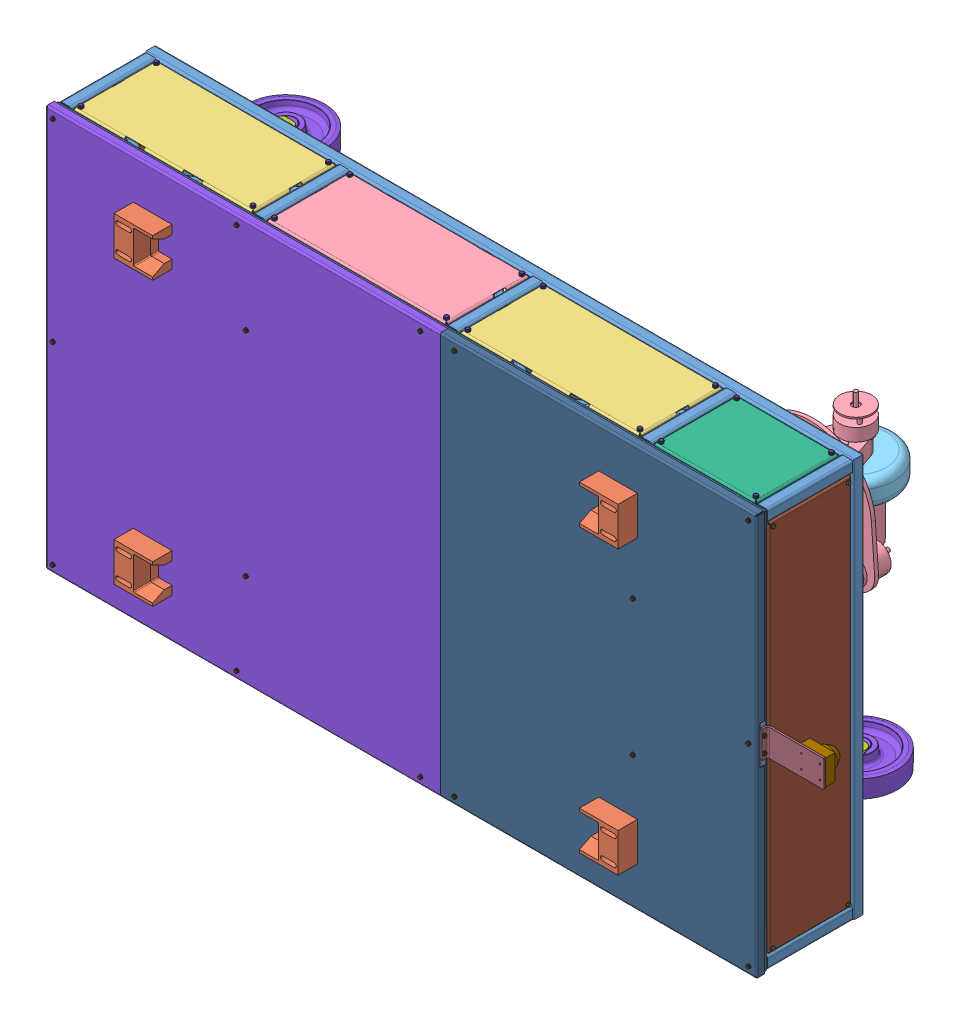
SolidWorks assembly spartaco_bot_V1, configuration Default. Lengths in mm.
Overall size (1986.1 1042.2 588.68).
206 component instances, 48 part files, 27 mates.
Components (placement in the parent):
- robot_body-1: robot_body [Default] at (-881.7629 -500.0018 -180.7451) x (0 -1 0) z (-1 0 0) size (1042.2 351.5 1986.1)
  - 00-A-PT0046 (1).step-1: 00-A-PT0046 (1).step [Default] at origin size (1042.2 306.3 1986.1)
    - 00-P-PT0151_Default_A macchina_.step-1: 00-P-PT0151_Default_A macchina_.step [Default] at origin size (1030 285 1830)
    - 00-P-PT0177.step-1: 00-P-PT0177.step [Default] at (-500 125 15) size (965 215 15)
    - 00-P-PT0153.step-1: 00-P-PT0153.step [Default] at (-1015 125 -250) x (0 0 1) z (-1 0 0) size (465 215 15)
    - 00-P-PT0153.step-2: 00-P-PT0153.step [Default] at (15 125 -250) x (0 0 -1) z (1 0 0) size (465 215 15)
    - 00-P-PT0153.step-3: 00-P-PT0153.step [Default] at (15 125 -1250) x (0 0 -1) z (1 0 0) size (465 215 15)
    - 00-P-PT0153.step-4: 00-P-PT0153.step [Default] at (-1015 125 -1250) x (0 0 1) z (-1 0 0) size (465 215 15)
    - 00-P-PT0169.step-1: 00-P-PT0169.step [Default] at (-1015 125 -750) x (0 0 1) z (-1 0 0) size (465 215 15)
    - 00-P-PT0154.step-1: 00-P-PT0154.step [Default] at (-500 -35 -750) x (0 0 1) z (-1 0 0) size (525 53 557)
    - 00-P-PT0168.step-1: 00-P-PT0168.step [Default] at (15 125 -1650) x (0 0 -1) z (1 0 0) size (265 215 15)
    - 00-P-PT0168.step-2: 00-P-PT0168.step [Default] at (-1015 125 -1650) x (0 0 1) z (-1 0 0) size (265 215 15)
    - 00-A-PT0167.step-1: 00-A-PT0167.step [Default] at (-500 -31 -590) size (500 35 45)
    - 00-P-PT0169.step-2: 00-P-PT0169.step [Default] at (15 125 -750) x (0 0 -1) z (1 0 0) size (465 215 15)
    - 00-A-PT0167.step-2: 00-A-PT0167.step [Default] at (-500 -31 -910) x (-1 0 0) z (0 0 -1) size (500 35 45)
    - 00-P-PT0174.step-1: 00-P-PT0174.step [Default] at (-500 266.5 -899.5) x (0 0 1) z (-1 0 0) size (1020 20 1038.01)
    - 00-P-PT0173.step-1: 00-P-PT0173.step [Default] at (-25 15 -990) x (0 0 1) z (1 0 0) size (500 2 950)
    - 00-P-PT0171.step-1: 00-P-PT0171.step [Default] at (-500 266.5 -899.5) x (0 0 -1) z (1 0 0) size (818 20 1038.01)
    - 00-p-pt0152.step-1: 00-p-pt0152.step [Default] at (-500 125 -1815) x (-1 0 0) z (0 0 -1) size (965 215 15)
    - 00-P-PT0175.step-1: 00-P-PT0175.step [Default] at (-25 17 -505) x (0 0 -1) z (1 0 0) size (190 2 950)
    - 00-p-pt0176.step-1: 00-p-pt0176.step [Default] at (-535 234.8 -1815) size (70 20 150)
    - Rosetta Piana UNI6592_130909006.step-1: Rosetta Piana UNI6592_130909006.step [Default] at (-1015.8 27.5 -1527.5) x (0 -1 0) z (0 0 1) size (11 1.6 11)
    - Rosetta Piana UNI6592_130909006.step-2: Rosetta Piana UNI6592_130909006.step [Default] at (-1015.8 222.5 -1527.5) x (0 -1 0) z (0 0 1) size (11 1.6 11)
    - Rosetta Piana UNI6592_130909006.step-3: Rosetta Piana UNI6592_130909006.step [Default] at (-1015.8 222.5 -1772.5) x (0 -1 0) z (0 0 1) size (11 1.6 11)
    - Rosetta Piana UNI6592_130909006.step-4: Rosetta Piana UNI6592_130909006.step [Default] at (-1015.8 27.5 -1772.5) x (0 -1 0) z (0 0 1) size (11 1.6 11)
    - Rosetta Piana UNI6592_130909006.step-5: Rosetta Piana UNI6592_130909006.step [Default] at (-1015.8 27.5 -1472.5) x (0 -1 0) z (0 0 1) size (11 1.6 11)
    - Rosetta Piana UNI6592_130909006.step-6: Rosetta Piana UNI6592_130909006.step [Default] at (-1015.8 27.5 -1027.5) x (0 0 -1) z (0 -1 0) size (11 1.6 11)
    - Rosetta Piana UNI6592_130909006.step-7: Rosetta Piana UNI6592_130909006.step [Default] at (-1015.8 222.5 -972.5) x (0 -1 0) z (0 0 1) size (11 1.6 11)
    - Rosetta Piana UNI6592_130909006.step-8: Rosetta Piana UNI6592_130909006.step [Default] at (-1015.8 222.5 -527.5) x (0 -1 0) z (0 0 1) size (11 1.6 11)
    - Rosetta Piana UNI6592_130909006.step-9: Rosetta Piana UNI6592_130909006.step [Default] at (-1015.8 27.5 -472.5) x (0 -1 0) z (0 0 1) size (11 1.6 11)
    - Rosetta Piana UNI6592_130909006.step-10: Rosetta Piana UNI6592_130909006.step [Default] at (-1015.8 27.5 -27.5) x (0 -1 0) z (0 0 1) size (11 1.6 11)
    - Rosetta Piana UNI6592_130909006.step-11: Rosetta Piana UNI6592_130909006.step [Default] at (-972.5 222.5 0.6) x (1 0 0) z (0 1 0) size (11 1.6 11)
    - Rosetta Piana UNI6592_130909006.step-12: Rosetta Piana UNI6592_130909006.step [Default] at (-972.5 27.5 15.8) x (1 0 0) z (0 1 0) size (11 1.6 11)
    - Rosetta Piana UNI6592_130909006.step-13: Rosetta Piana UNI6592_130909006.step [Default] at (-27.5 27.5 15.8) x (1 0 0) z (0 1 0) size (11 1.6 11)
    - Rosetta Piana UNI6592_130909006.step-14: Rosetta Piana UNI6592_130909006.step [Default] at (15.8 27.5 -27.5) x (0 1 0) z (0 0 1) size (11 1.6 11)
    - Rosetta Piana UNI6592_130909006.step-15: Rosetta Piana UNI6592_130909006.step [Default] at (15.8 27.5 -472.5) x (0 1 0) z (0 0 1) size (11 1.6 11)
    - Rosetta Piana UNI6592_130909006.step-16: Rosetta Piana UNI6592_130909006.step [Default] at (15.8 222.5 -527.5) x (0 1 0) z (0 0 1) size (11 1.6 11)
    - Rosetta Piana UNI6592_130909006.step-17: Rosetta Piana UNI6592_130909006.step [Default] at (15.8 222.5 -972.5) x (0 1 0) z (0 0 1) size (11 1.6 11)
    - Rosetta Piana UNI6592_130909006.step-18: Rosetta Piana UNI6592_130909006.step [Default] at (15.8 27.5 -1027.5) x (0 1 0) z (0 0 1) size (11 1.6 11)
    - Rosetta Piana UNI6592_130909006.step-19: Rosetta Piana UNI6592_130909006.step [Default] at (15.8 27.5 -1472.5) x (0 1 0) z (0 0 1) size (11 1.6 11)
    - Rosetta Piana UNI6592_130909006.step-20: Rosetta Piana UNI6592_130909006.step [Default] at (15.8 27.5 -1527.5) x (0 1 0) z (0 0 1) size (11 1.6 11)
    - Rosetta Piana UNI6592_130909006.step-21: Rosetta Piana UNI6592_130909006.step [Default] at (15.8 27.5 -1772.5) x (0 1 0) z (0 0 1) size (11 1.6 11)
    - Rosetta Piana UNI6592_130909006.step-22: Rosetta Piana UNI6592_130909006.step [Default] at (15.8 222.5 -1527.5) x (0 1 0) z (0 0 1) size (11 1.6 11)
    - Rosetta Piana UNI6592_130909006.step-23: Rosetta Piana UNI6592_130909006.step [Default] at (15.8 222.5 -1772.5) x (0 1 0) z (0 0 1) size (11 1.6 11)
    - Rosetta Piana UNI6592_130909005.step-1: Rosetta Piana UNI6592_130909005.step [Default] at (-27.5 27.5 -1815.4) x (1 0 0) z (0 -1 0) size (10 0.8 10)
    - Rosetta Piana UNI6592_130909005.step-2: Rosetta Piana UNI6592_130909005.step [Default] at (-27.5 222.5 -1815.4) x (1 0 0) z (0 -1 0) size (10 0.8 10)
    - Rosetta Piana UNI6592_130909005.step-3: Rosetta Piana UNI6592_130909005.step [Default] at (-972.5 27.5 -1815.4) x (1 0 0) z (0 -1 0) size (10 0.8 10)
    - Rosetta Piana UNI6592_130909005.step-4: Rosetta Piana UNI6592_130909005.step [Default] at (-972.5 222.5 -1815.4) x (1 0 0) z (0 -1 0) size (10 0.8 10)
    - Rosetta Piana UNI6592_130909005.step-5: Rosetta Piana UNI6592_130909005.step [Default] at (-750 18.4 -500) x (0.837169 0 0.546944) z (0.546944 0 -0.837169) size (10 0.8 10)
    - Rosetta Piana UNI6592_130909005.step-6: Rosetta Piana UNI6592_130909005.step [Default] at (-500 18.4 -500) x (0.837169 0 0.546944) z (0.546944 0 -0.837169) size (10 0.8 10)
    - Rosetta Piana UNI6592_130909005.step-7: Rosetta Piana UNI6592_130909005.step [Default] at (-250 18.4 -500) x (0.837169 0 0.546944) z (0.546944 0 -0.837169) size (10 0.8 10)
    - Rosetta Piana UNI6592_130909005.step-8: Rosetta Piana UNI6592_130909005.step [Default] at (-250 18.4 -1000) x (0.837169 0 0.546944) z (0.546944 0 -0.837169) size (10 0.8 10)
    - Rosetta Piana UNI6592_130909005.step-9: Rosetta Piana UNI6592_130909005.step [Default] at (-500 18.4 -1000) x (0.837169 0 0.546944) z (0.546944 0 -0.837169) size (10 0.8 10)
    - Rosetta Piana UNI6592_130909005.step-10: Rosetta Piana UNI6592_130909005.step [Default] at (-750 18.4 -1000) x (0.837169 0 0.546944) z (0.546944 0 -0.837169) size (10 0.8 10)
    - V.T.E. Zinc UNI 5739_130328056.step-1: V.T.E. Zinc UNI 5739_130328056.step [Default] at (-750 19.3 -500) size (9.24 24 9.25)
    - V.T.E. Zinc UNI 5739_130328056.step-2: V.T.E. Zinc UNI 5739_130328056.step [Default] at (-500 19.3 -500) size (9.24 24 9.25)
    - V.T.E. Zinc UNI 5739_130328056.step-3: V.T.E. Zinc UNI 5739_130328056.step [Default] at (-250 19.3 -500) size (9.24 24 9.25)
    - V.T.E. Zinc UNI 5739_130328056.step-4: V.T.E. Zinc UNI 5739_130328056.step [Default] at (-250 19.3 -1000) size (9.24 24 9.25)
    - V.T.E. Zinc UNI 5739_130328056.step-5: V.T.E. Zinc UNI 5739_130328056.step [Default] at (-500 19.3 -1000) size (9.24 24 9.25)
    - V.T.E. Zinc UNI 5739_130328056.step-6: V.T.E. Zinc UNI 5739_130328056.step [Default] at (-750 19.3 -1000) size (9.24 24 9.25)
    - Rosetta Piana UNI6592_130909006.step-24: Rosetta Piana UNI6592_130909006.step [Default] at (15.8 222.5 -27.5) x (0 1 0) z (0 0 1) size (11 1.6 11)
    - Rosetta Piana UNI6592_130909006.step-25: Rosetta Piana UNI6592_130909006.step [Default] at (15.8 222.5 -472.5) x (0 1 0) z (0 0 1) size (11 1.6 11)
    - Rosetta Piana UNI6592_130909006.step-26: Rosetta Piana UNI6592_130909006.step [Default] at (15.8 27.5 -527.5) x (0 1 0) z (0 0 1) size (11 1.6 11)
    - Rosetta Piana UNI6592_130909006.step-27: Rosetta Piana UNI6592_130909006.step [Default] at (15.8 27.5 -972.5) x (0 1 0) z (0 0 1) size (11 1.6 11)
    - Rosetta Piana UNI6592_130909006.step-28: Rosetta Piana UNI6592_130909006.step [Default] at (15.8 222.5 -1027.5) x (0 1 0) z (0 0 1) size (11 1.6 11)
    - Rosetta Piana UNI6592_130909006.step-29: Rosetta Piana UNI6592_130909006.step [Default] at (15.8 222.5 -1472.5) x (0 1 0) z (0 0 1) size (11 1.6 11)
    - Rosetta Piana UNI6592_130909006.step-30: Rosetta Piana UNI6592_130909006.step [Default] at (-1015.8 222.5 -1472.5) x (0 -1 0) z (0 0 1) size (11 1.6 11)
    - Rosetta Piana UNI6592_130909006.step-31: Rosetta Piana UNI6592_130909006.step [Default] at (-1015.8 222.5 -1027.5) x (0 -1 0) z (0 0 1) size (11 1.6 11)
    - Rosetta Piana UNI6592_130909006.step-32: Rosetta Piana UNI6592_130909006.step [Default] at (-1015.8 27.5 -972.5) x (0 -1 0) z (0 0 1) size (11 1.6 11)
    - Rosetta Piana UNI6592_130909006.step-33: Rosetta Piana UNI6592_130909006.step [Default] at (-1015.8 27.5 -527.5) x (0 -1 0) z (0 0 1) size (11 1.6 11)
    - Rosetta Piana UNI6592_130909006.step-34: Rosetta Piana UNI6592_130909006.step [Default] at (-1015.8 222.5 -472.5) x (0 -1 0) z (0 0 1) size (11 1.6 11)
    - Rosetta Piana UNI6592_130909006.step-35: Rosetta Piana UNI6592_130909006.step [Default] at (-1015.8 222.5 -27.5) x (0 -1 0) z (0 0 1) size (11 1.6 11)
    - Rosetta Piana UNI6592_130909005.step-11: Rosetta Piana UNI6592_130909005.step [Default] at (-1 266.9 -0.5) x (0.837169 0 0.546944) z (0.546944 0 -0.837169) size (10 0.8 10)
    - Rosetta Piana UNI6592_130909005.step-12: Rosetta Piana UNI6592_130909005.step [Default] at (-1 266.9 -475.5) x (0.837169 0 0.546944) z (0.546944 0 -0.837169) size (10 0.8 10)
    - Rosetta Piana UNI6592_130909005.step-13: Rosetta Piana UNI6592_130909005.step [Default] at (-500 266.9 -0.5) x (0.837169 0 0.546944) z (0.546944 0 -0.837169) size (10 0.8 10)
    - Rosetta Piana UNI6592_130909005.step-14: Rosetta Piana UNI6592_130909005.step [Default] at (-225 266.9 -499.5) x (0.837169 0 0.546944) z (0.546944 0 -0.837169) size (10 0.8 10)
    - Rosetta Piana UNI6592_130909005.step-15: Rosetta Piana UNI6592_130909005.step [Default] at (-775 266.9 -499.5) x (0.837169 0 0.546944) z (0.546944 0 -0.837169) size (10 0.8 10)
    - Rosetta Piana UNI6592_130909005.step-16: Rosetta Piana UNI6592_130909005.step [Default] at (-999 266.9 -475.5) x (0.837169 0 0.546944) z (0.546944 0 -0.837169) size (10 0.8 10)
    - Rosetta Piana UNI6592_130909005.step-17: Rosetta Piana UNI6592_130909005.step [Default] at (-999 266.9 -0.5) x (0.837169 0 0.546944) z (0.546944 0 -0.837169) size (10 0.8 10)
    - Rosetta Piana UNI6592_130909005.step-18: Rosetta Piana UNI6592_130909005.step [Default] at (-1 266.9 -950.5) x (0.837169 0 0.546944) z (0.546944 0 -0.837169) size (10 0.8 10)
    - Rosetta Piana UNI6592_130909005.step-19: Rosetta Piana UNI6592_130909005.step [Default] at (-1 266.9 -1038.5) x (0.837169 0 0.546944) z (0.546944 0 -0.837169) size (10 0.8 10)
    - Rosetta Piana UNI6592_130909005.step-20: Rosetta Piana UNI6592_130909005.step [Default] at (-325 266.9 -1500) x (0.837169 0 0.546944) z (0.546944 0 -0.837169) size (10 0.8 10)
    - Rosetta Piana UNI6592_130909005.step-21: Rosetta Piana UNI6592_130909005.step [Default] at (-1 266.9 -1798.5) x (0.837169 0 0.546944) z (0.546944 0 -0.837169) size (10 0.8 10)
    - Rosetta Piana UNI6592_130909005.step-22: Rosetta Piana UNI6592_130909005.step [Default] at (-500 266.9 -1798.5) x (0.837169 0 0.546944) z (0.546944 0 -0.837169) size (10 0.8 10)
    - Rosetta Piana UNI6592_130909005.step-23: Rosetta Piana UNI6592_130909005.step [Default] at (-675 266.9 -1500) x (0.837169 0 0.546944) z (0.546944 0 -0.837169) size (10 0.8 10)
    - Rosetta Piana UNI6592_130909005.step-24: Rosetta Piana UNI6592_130909005.step [Default] at (-999 266.9 -1798.5) x (0.837169 0 0.546944) z (0.546944 0 -0.837169) size (10 0.8 10)
    - Rosetta Piana UNI6592_130909005.step-25: Rosetta Piana UNI6592_130909005.step [Default] at (-999 266.9 -1038.5) x (0.837169 0 0.546944) z (0.546944 0 -0.837169) size (10 0.8 10)
    - Rosetta Piana UNI6592_130909005.step-26: Rosetta Piana UNI6592_130909005.step [Default] at (-999 266.9 -950.5) x (0.837169 0 0.546944) z (0.546944 0 -0.837169) size (10 0.8 10)
    - Rosetta Piana UNI6592_130909005.step-27: Rosetta Piana UNI6592_130909005.step [Default] at (-480 249.8 -1820.4) x (1 0 0) z (0 -1 0) size (10 0.8 10)
    - Rosetta Piana UNI6592_130909005.step-28: Rosetta Piana UNI6592_130909005.step [Default] at (-520 249.8 -1820.4) x (1 0 0) z (0 -1 0) size (10 0.8 10)
    - V.T.E. Zinc UNI 5739_130328089.step-1: V.T.E. Zinc UNI 5739_130328089.step [Default] at (-1017.1 222.5 -1772.5) x (0 1 0) z (0 0 1) size (11.56 34.5 11.57)
    - V.T.E. Zinc UNI 5739_130328089.step-2: V.T.E. Zinc UNI 5739_130328089.step [Default] at (-1017.1 222.5 -1527.5) x (0 1 0) z (0 0 1) size (11.56 34.5 11.57)
    - V.T.E. Zinc UNI 5739_130328089.step-3: V.T.E. Zinc UNI 5739_130328089.step [Default] at (-1017.1 27.5 -1772.5) x (0 1 0) z (0 0 1) size (11.56 34.5 11.57)
    - V.T.E. Zinc UNI 5739_130328089.step-4: V.T.E. Zinc UNI 5739_130328089.step [Default] at (-1017.1 27.5 -1527.5) x (0 1 0) z (0 0 1) size (11.56 34.5 11.57)
    - V.T.E. Zinc UNI 5739_130328089.step-5: V.T.E. Zinc UNI 5739_130328089.step [Default] at (-1017.1 27.5 -1472.5) x (0 1 0) z (0 0 1) size (11.56 34.5 11.57)
    - V.T.E. Zinc UNI 5739_130328089.step-6: V.T.E. Zinc UNI 5739_130328089.step [Default] at (-1017.1 27.5 -1027.5) x (0 1 0) z (0 0 1) size (11.56 34.5 11.57)
    - V.T.E. Zinc UNI 5739_130328089.step-7: V.T.E. Zinc UNI 5739_130328089.step [Default] at (-1017.1 222.5 -972.5) x (0 1 0) z (0 0 1) size (11.56 34.5 11.57)
    - V.T.E. Zinc UNI 5739_130328089.step-8: V.T.E. Zinc UNI 5739_130328089.step [Default] at (-1017.1 222.5 -527.5) x (0 1 0) z (0 0 1) size (11.56 34.5 11.57)
    - V.T.E. Zinc UNI 5739_130328089.step-9: V.T.E. Zinc UNI 5739_130328089.step [Default] at (-1017.1 27.5 -472.5) x (0 1 0) z (0 0 1) size (11.56 34.5 11.57)
    - V.T.E. Zinc UNI 5739_130328089.step-10: V.T.E. Zinc UNI 5739_130328089.step [Default] at (-1017.1 27.5 -27.5) x (0 1 0) z (0 0 1) size (11.56 34.5 11.57)
    - V.T.E. Zinc UNI 5739_130328089.step-11: V.T.E. Zinc UNI 5739_130328089.step [Default] at (-972.5 27.5 17.1) x (1 0 0) z (0 -1 0) size (11.56 34.5 11.57)
    - V.T.E. Zinc UNI 5739_130328089.step-12: V.T.E. Zinc UNI 5739_130328089.step [Default] at (-27.5 27.5 17.1) x (1 0 0) z (0 -1 0) size (11.56 34.5 11.57)
    - V.T.E. Zinc UNI 5739_130328089.step-13: V.T.E. Zinc UNI 5739_130328089.step [Default] at (17.1 27.5 -27.5) x (0 -1 0) z (0 0 1) size (11.56 34.5 11.57)
    - V.T.E. Zinc UNI 5739_130328089.step-14: V.T.E. Zinc UNI 5739_130328089.step [Default] at (17.1 27.5 -472.5) x (0 -1 0) z (0 0 1) size (11.56 34.5 11.57)
    - V.T.E. Zinc UNI 5739_130328089.step-15: V.T.E. Zinc UNI 5739_130328089.step [Default] at (17.1 222.5 -527.5) x (0 -1 0) z (0 0 1) size (11.56 34.5 11.57)
    - V.T.E. Zinc UNI 5739_130328089.step-16: V.T.E. Zinc UNI 5739_130328089.step [Default] at (17.1 222.5 -972.5) x (0 -1 0) z (0 0 1) size (11.56 34.5 11.57)
    - V.T.E. Zinc UNI 5739_130328089.step-17: V.T.E. Zinc UNI 5739_130328089.step [Default] at (17.1 27.5 -1027.5) x (0 -1 0) z (0 0 1) size (11.56 34.5 11.57)
    - V.T.E. Zinc UNI 5739_130328089.step-18: V.T.E. Zinc UNI 5739_130328089.step [Default] at (17.1 27.5 -1472.5) x (0 -1 0) z (0 0 1) size (11.56 34.5 11.57)
    - V.T.E. Zinc UNI 5739_130328089.step-19: V.T.E. Zinc UNI 5739_130328089.step [Default] at (17.1 27.5 -1527.5) x (0 -1 0) z (0 0 1) size (11.56 34.5 11.57)
    - V.T.E. Zinc UNI 5739_130328089.step-20: V.T.E. Zinc UNI 5739_130328089.step [Default] at (17.1 27.5 -1772.5) x (0 -1 0) z (0 0 1) size (11.56 34.5 11.57)
    - V.T.E. Zinc UNI 5739_130328089.step-21: V.T.E. Zinc UNI 5739_130328089.step [Default] at (17.1 222.5 -1527.5) x (0 -1 0) z (0 0 1) size (11.56 34.5 11.57)
    - V.T.E. Zinc UNI 5739_130328089.step-22: V.T.E. Zinc UNI 5739_130328089.step [Default] at (17.1 222.5 -1772.5) x (0 -1 0) z (0 0 1) size (11.56 34.5 11.57)
    - Rosetta Piana UNI6592_130909006.step-36: Rosetta Piana UNI6592_130909006.step [Default] at (-972.5 222.5 15.8) x (1 0 0) z (0 1 0) size (11 1.6 11)
    - Rosetta Piana UNI6592_130909006.step-37: Rosetta Piana UNI6592_130909006.step [Default] at (-27.5 222.5 15.8) x (1 0 0) z (0 1 0) size (11 1.6 11)
    - V.T.E. Zinc UNI 5739_130328089.step-23: V.T.E. Zinc UNI 5739_130328089.step [Default] at (-27.5 222.5 17.1) x (1 0 0) z (0 -1 0) size (11.56 34.5 11.57)
    - V.T.E. Zinc UNI 5739_130328089.step-24: V.T.E. Zinc UNI 5739_130328089.step [Default] at (-972.5 222.5 17.1) x (1 0 0) z (0 -1 0) size (11.56 34.5 11.57)
    - V.T.E. Zinc UNI 5739_130328056.step-7: V.T.E. Zinc UNI 5739_130328056.step [Default] at (-27.5 27.5 -1816.3) x (0.960124 0.279576 0) z (-0.279576 0.960124 0) size (9.24 24 9.25)
    - V.T.E. Zinc UNI 5739_130328056.step-8: V.T.E. Zinc UNI 5739_130328056.step [Default] at (-27.5 222.5 -1816.3) x (-0.948121 0.317909 0) z (-0.317909 -0.948121 0) size (9.24 24 9.25)
    - V.T.E. Zinc UNI 5739_130328056.step-9: V.T.E. Zinc UNI 5739_130328056.step [Default] at (-972.5 27.5 -1816.3) x (1 0 0) z (0 1 0) size (9.24 24 9.25)
    - V.T.E. Zinc UNI 5739_130328056.step-10: V.T.E. Zinc UNI 5739_130328056.step [Default] at (-972.5 222.5 -1816.3) x (1 0 0) z (0 1 0) size (9.24 24 9.25)
    - V.T.E. Zinc UNI 5739_130328089.step-25: V.T.E. Zinc UNI 5739_130328089.step [Default] at (17.1 222.5 -27.5) x (0 -1 0) z (0 0 1) size (11.56 34.5 11.57)
    - V.T.E. Zinc UNI 5739_130328089.step-26: V.T.E. Zinc UNI 5739_130328089.step [Default] at (17.1 222.5 -472.5) x (0 -1 0) z (0 0 1) size (11.56 34.5 11.57)
    - V.T.E. Zinc UNI 5739_130328089.step-27: V.T.E. Zinc UNI 5739_130328089.step [Default] at (17.1 27.5 -527.5) x (0 -1 0) z (0 0 1) size (11.56 34.5 11.57)
    - V.T.E. Zinc UNI 5739_130328089.step-28: V.T.E. Zinc UNI 5739_130328089.step [Default] at (17.1 27.5 -972.5) x (0 -1 0) z (0 0 1) size (11.56 34.5 11.57)
    - V.T.E. Zinc UNI 5739_130328089.step-29: V.T.E. Zinc UNI 5739_130328089.step [Default] at (17.1 222.5 -1027.5) x (0 -1 0) z (0 0 1) size (11.56 34.5 11.57)
    - V.T.E. Zinc UNI 5739_130328089.step-30: V.T.E. Zinc UNI 5739_130328089.step [Default] at (17.1 222.5 -1472.5) x (0 -1 0) z (0 0 1) size (11.56 34.5 11.57)
    - V.T.E. Zinc UNI 5739_130328089.step-31: V.T.E. Zinc UNI 5739_130328089.step [Default] at (-1017.1 222.5 -1472.5) x (0 1 0) z (0 0 1) size (11.56 34.5 11.57)
    - V.T.E. Zinc UNI 5739_130328089.step-32: V.T.E. Zinc UNI 5739_130328089.step [Default] at (-1017.1 222.5 -1027.5) x (0 1 0) z (0 0 1) size (11.56 34.5 11.57)
    - V.T.E. Zinc UNI 5739_130328089.step-33: V.T.E. Zinc UNI 5739_130328089.step [Default] at (-1017.1 27.5 -527.5) x (0 1 0) z (0 0 1) size (11.56 34.5 11.57)
    - V.T.E. Zinc UNI 5739_130328089.step-34: V.T.E. Zinc UNI 5739_130328089.step [Default] at (-1017.1 222.5 -472.5) x (0 1 0) z (0 0 1) size (11.56 34.5 11.57)
    - V.T.E. Zinc UNI 5739_130328089.step-35: V.T.E. Zinc UNI 5739_130328089.step [Default] at (-1017.1 222.5 -27.5) x (0 1 0) z (0 0 1) size (11.56 34.5 11.57)
    - V.T.E. Zinc UNI 5739_130328089.step-36: V.T.E. Zinc UNI 5739_130328089.step [Default] at (-1017.1 27.5 -972.5) x (0 1 0) z (0 0 1) size (11.56 34.5 11.57)
    - V.T.E. Zinc UNI 5739 M5_Vite TE M5X16.step-1: V.T.E. Zinc UNI 5739 M5_Vite TE M5X16.step [Default] at (-1 267.8 -0.5) size (9.24 20 9.25)
    - V.T.E. Zinc UNI 5739 M5_Vite TE M5X16.step-2: V.T.E. Zinc UNI 5739 M5_Vite TE M5X16.step [Default] at (-500 267.8 -0.5) size (9.24 20 9.25)
    - V.T.E. Zinc UNI 5739 M5_Vite TE M5X16.step-3: V.T.E. Zinc UNI 5739 M5_Vite TE M5X16.step [Default] at (-225 267.8 -499.5) size (9.24 20 9.25)
    - V.T.E. Zinc UNI 5739 M5_Vite TE M5X16.step-4: V.T.E. Zinc UNI 5739 M5_Vite TE M5X16.step [Default] at (-1 267.8 -475.5) size (9.24 20 9.25)
    - V.T.E. Zinc UNI 5739 M5_Vite TE M5X16.step-5: V.T.E. Zinc UNI 5739 M5_Vite TE M5X16.step [Default] at (-1 267.8 -950.5) size (9.24 20 9.25)
    - V.T.E. Zinc UNI 5739 M5_Vite TE M5X16.step-6: V.T.E. Zinc UNI 5739 M5_Vite TE M5X16.step [Default] at (-1 267.8 -1038.5) size (9.24 20 9.25)
    - V.T.E. Zinc UNI 5739 M5_Vite TE M5X16.step-7: V.T.E. Zinc UNI 5739 M5_Vite TE M5X16.step [Default] at (-1 267.8 -1798.5) size (9.24 20 9.25)
    - V.T.E. Zinc UNI 5739 M5_Vite TE M5X16.step-8: V.T.E. Zinc UNI 5739 M5_Vite TE M5X16.step [Default] at (-325 267.8 -1500) size (9.24 20 9.25)
    - V.T.E. Zinc UNI 5739 M5_Vite TE M5X16.step-9: V.T.E. Zinc UNI 5739 M5_Vite TE M5X16.step [Default] at (-500 267.8 -1798.5) size (9.24 20 9.25)
    - V.T.E. Zinc UNI 5739 M5_Vite TE M5X16.step-10: V.T.E. Zinc UNI 5739 M5_Vite TE M5X16.step [Default] at (-675 267.8 -1500) size (9.24 20 9.25)
    - V.T.E. Zinc UNI 5739 M5_Vite TE M5X16.step-11: V.T.E. Zinc UNI 5739 M5_Vite TE M5X16.step [Default] at (-999 267.8 -1798.5) size (9.24 20 9.25)
    - V.T.E. Zinc UNI 5739 M5_Vite TE M5X16.step-12: V.T.E. Zinc UNI 5739 M5_Vite TE M5X16.step [Default] at (-999 267.8 -1038.5) size (9.24 20 9.25)
    - V.T.E. Zinc UNI 5739 M5_Vite TE M5X16.step-13: V.T.E. Zinc UNI 5739 M5_Vite TE M5X16.step [Default] at (-999 267.8 -950.5) size (9.24 20 9.25)
    - V.T.E. Zinc UNI 5739 M5_Vite TE M5X16.step-14: V.T.E. Zinc UNI 5739 M5_Vite TE M5X16.step [Default] at (-999 267.8 -0.5) size (9.24 20 9.25)
    - V.T.E. Zinc UNI 5739 M5_Vite TE M5X16.step-15: V.T.E. Zinc UNI 5739 M5_Vite TE M5X16.step [Default] at (-480 249.8 -1821.3) x (1 0 0) z (0 1 0) size (9.24 20 9.25)
    - V.T.E. Zinc UNI 5739 M5_Vite TE M5X16.step-16: V.T.E. Zinc UNI 5739 M5_Vite TE M5X16.step [Default] at (-520 249.8 -1821.3) x (1 0 0) z (0 1 0) size (9.24 20 9.25)
    - V.T.E. Zinc UNI 5739 M5_Vite TE M5X16.step-17: V.T.E. Zinc UNI 5739 M5_Vite TE M5X16.step [Default] at (-999 267.8 -475.5) size (9.24 20 9.25)
    - V.T.E. Zinc UNI 5739 M5_Vite TE M5X16.step-18: V.T.E. Zinc UNI 5739 M5_Vite TE M5X16.step [Default] at (-775 267.8 -499.5) size (9.24 20 9.25)
    - 00-P-PT0178.step-1: 00-P-PT0178.step [Default] at (-500 17 -1015) x (0 0 -1) z (1 0 0) size (50 240 600)
  - cuneo_pedana-1: cuneo_pedana [Default] at (-865 266.5 -207) size (100 50 100)
  - cuneo_pedana-2: cuneo_pedana [Default] at (-135 266.5 -1510) x (-1 0 0) z (0 0 -1) size (100 50 100)
  - cuneo_pedana-3: cuneo_pedana [Default] at (-865 266.5 -1510) x (-1 0 0) z (0 0 -1) size (100 50 100)
  - cuneo_pedana-4: cuneo_pedana [Default] at (-135 266.5 -207) size (100 50 100)
- batteria-1: batteria [Default] at (-131.7629 -0.0018 -212.7451) x (0 -1 0) z (-1 0 0) size (569 275 320)
- MRT05-1: MRT05 [Default] at (-737.9796 -364.3122 -288.3365) x (-1 0 0) z (0 1 0) size (337.24 246.99 360.81)
  - MRT05-1: MRT05 [Default] at (-16.2167 -3.4086 117.2864) x (-1 0 0) z (0 0 -1) size (337.24 211.1 360.81)
  - MRT05_wheel-1: MRT05_wheel [Default] at (-16.2167 -60.4032 39.3104) x (0 0 1) z (-1 0 0) size (71 198 198)
- MRT05-2: MRT05 [Default] at (742.0204 285.6878 -288.3365) x (-1 0 0) z (0 1 0) size (337.24 246.99 360.81)
  - MRT05-1: MRT05 [Default] at (-16.2167 -3.4086 117.2864) x (-1 0 0) z (0 0 -1) size (337.24 211.1 360.81)
  - MRT05_wheel-1: MRT05_wheel [Default] at (-16.2167 -60.4032 39.3104) x (0 0 1) z (-1 0 0) size (71 198 198)
- castor_pivot-1: castor_pivot [Default] at (823.2371 -325.0018 -210.5605) x (1 0 0) z (0 0 -1) size (204.58 110 156.49)
  - piastra_pivot-1: piastra_pivot [Default] at (0 0 -9.8154) size (135 110 24.79)
  - pivot-1: pivot [Default] at (-57.8 -35.5 138.1746) x (1 0 0) z (0 1 0) size (183.58 152.49 93)
- castor_pivot-2: castor_pivot [Default] at (-656.7629 324.9982 -210.5605) x (1 0 0) z (0 0 -1) size (204.58 110 156.49)
  - piastra_pivot-1: piastra_pivot [Default] at (0 0 -9.8154) size (135 110 24.79)
  - pivot-1: pivot [Default] at (-57.8 -35.5 138.1746) x (1 0 0) z (0 1 0) size (183.58 152.49 93)
- wheel_200-1: wheel_200 [Default] at (-714.5629 324.9982 -348.7351) x (0 1 0) z (1 0 0) size (62.5 200 200)
- wheel_200-2: wheel_200 [Default] at (765.4371 -325.0018 -348.7351) x (0 1 0) z (0.999085 0 0.042769) size (62.5 200 200)
- lidar-1: lidar [Default] at (1049.2371 -0.0018 54.0549) x (-1 0 0) z (0 0 -1) size (73 65 60)
- quadro_elettrico_full-1: quadro_elettrico_full [Default] at (403.2371 -0.0018 -163.7451) x (0 1 0) z (0 0 1) size (930 400 160)
  - quadro_elettrico-1: quadro_elettrico [Default] at origin size (930 400 160)
  - minitraction_power_mockup-1: minitraction_power_mockup [Default] at (67.5 -105 10) size (85 130 40)
  - SD-100C-12-1: SD-100C-12 [Default] at (-124.5 -91.125 11.5) x (1 0 0) z (0 -1 0) size (199.09 37.75 98.27)
    - SD-100C-12.stp-1: SD-100C-12.stp [Default] at origin size (199.09 37.75 98.27)
      - SD-100-20201028.stp.stp-1: SD-100-20201028.stp.stp [Default] at origin size (199.09 37.75 98.27)
        - SD-100_STP.ASM.stp-1: SD-100_STP.ASM.stp [Default] at origin size (199.09 37.75 98.27)
          - SD-100_1_ASM.ASM.stp-1: SD-100_1_ASM.ASM.stp [Default] at origin size (199 37.75 98.27)
            - 902-D-80_ASM.ASM.stp-1: 902-D-80_ASM.ASM.stp [Default] at origin size (199 37.75 97.75)
              - 902-D-119_PRT.PRT.stp-1: 902-D-119_PRT.PRT.stp [Default] at origin size (199 37.75 97.75)
              - NUT_PRT.PRT.stp-1: NUT_PRT.PRT.stp [Default] at (-111.528 -1.5 -40.7894) x (-1 0 0) z (0 1 0) size (8 6.93 6)
            - 902-T_PRT.PRT.stp-1: 902-T_PRT.PRT.stp [Default] at (96.5 36.1 -49.375) x (-1 0 0) z (0 0 -1) size (195.5 36.02 96.52)
            - MYLAR_PRT.PRT.stp-1: MYLAR_PRT.PRT.stp [Default] at (79.2081 1.5 46.5396) x (-1 0 0) z (0 -1 0) size (197 95 0.5)
            - HS2_PRT.PRT.stp-1: HS2_PRT.PRT.stp [Default] at (-64.5 -80.2586 -88.3567) x (0 0 1) z (-1 0 0) size (6.4 28 55)
            - PCB_PRT.PRT.stp-1: PCB_PRT.PRT.stp [Default] at (-189.5595 4.5 45.0362) x (1 0 0) z (0 1 0) size (194 95 1.6)
          - T44-BS1R05370120201023_STP.ASM.stp-1: T44-BS1R05370120201023_STP.ASM.stp [Default] at (-82.3888 6.1 -32.875) x (0 0 1) z (0 1 0) size (69.8 18 18.8)
            - 6_PRT.PRT.stp-1: 6_PRT.PRT.stp [Default] at origin size (7.51 7.5 3.96)
            - 2_PRT.PRT.stp-1: 2_PRT.PRT.stp [Default] at origin size (7.5 7.5 3.96)
            - 3_PRT.PRT.stp-1: 3_PRT.PRT.stp [Default] at origin size (7.51 7.5 3.96)
            - 4_PRT.PRT.stp-1: 4_PRT.PRT.stp [Default] at (0 0.8 0) size (69.8 18 18.8)
            - 5_PRT.PRT.stp-1: 5_PRT.PRT.stp [Default] at origin size (7.51 7.5 3.96)
            - 6_PRT_1.PRT.stp-1: 6_PRT_1.PRT.stp [Default] at (9.5 0 0) size (7.51 7.5 3.96)
            - 6_PRT_1_1.PRT.stp-1: 6_PRT_1_1.PRT.stp [Default] at (19 0 0) size (7.51 7.5 3.96)
            - 6_PRT_1_1_1.PRT.stp-1: 6_PRT_1_1_1.PRT.stp [Default] at (28.5 0 0) size (7.51 7.5 3.96)
  - SD-25C-12-1: SD-25C-12 [Default] at (-36.8335 -327.0246 17.8) size (99.05 97.03 36.06)
    - SD-25C-12.stp-1: SD-25C-12.stp [Default] at origin size (99.05 97.03 36.06)
      - RS-50_ASM_15.ASM.stp-1: RS-50_ASM_15.ASM.stp [Default] at origin size (99.05 97.03 36.06)
        - TN1_2.PRT.stp-1: TN1_2.PRT.stp [Default] at (-301.0065 335.8998 37.1723) x (0 0 -1) z (-1 0 0) size (15.25 49.25 14.66)
        - RS-50-CASE-T_21.PRT.stp-1: RS-50-CASE-T_21.PRT.stp [Default] at (0 1.5 1) size (97.05 96.6 36.06)
        - RS-50-CASE-D_28.PRT.stp-1: RS-50-CASE-D_28.PRT.stp [Default] at (-0.5 0.5 0) size (98.5 97 35)
        - RS-50-PCB_2.PRT.stp-1: RS-50-PCB_2.PRT.stp [Default] at (0 -0.6 -0.2033) size (98 95 1.6)
  - minitraction_power_mockup-2: minitraction_power_mockup [Default] at (172.5 -105 10) size (85 130 40)
  - minitraction_power_mockup-3: minitraction_power_mockup [Default] at (277.5 -105 10) size (85 130 40)
  - minitraction_power_mockup-4: minitraction_power_mockup [Default] at (382.5 -105 10) size (85 130 40)
- panda_mockup-1: panda_mockup [Default] at (171.9371 -410.0018 -83.7451) x (0 1 0) z (1 0 0) size (110 160 39.6)
Mates (geometry in assembly coordinates):
- Coincidente1: coordinate: unknown of robot_body-1
- Coincidente2: coincident anti-aligned: plane of robot_body-1/00-A-PT0046 (1).step-1/00-P-PT0154.step-1 through (100.7371 272.4982 -212.7451) normal (0 0 1); plane of batteria-1 through (-131.7629 -0.0018 -212.7451) normal (0 0 -1)
- Larghezza1: width aligned: plane of robot_body-1/00-A-PT0046 (1).step-1/00-P-PT0154.step-1 through (-131.7629 275.4982 -215.7451) normal (0 -1 0); plane of batteria-1 through (-131.7629 -275.5018 -215.7451) normal (0 1 0); plane of robot_body-1/00-A-PT0046 (1).step-1/00-P-PT0154.step-1 through (-291.7629 -270.5018 62.2549) normal (0 -1 0); plane of batteria-1 through (-291.7629 270.4982 62.2549) normal (0 1 0)
- Larghezza2: width anti-aligned: plane of robot_body-1/00-A-PT0046 (1).step-1/00-A-PT0167.step-2 through (28.2371 249.9982 -176.7451) normal (-1 0 0); plane of batteria-1 through (-291.7629 -250.0018 -176.7451) normal (1 0 0); plane of robot_body-1/00-A-PT0046 (1).step-1/00-A-PT0167.step-1 through (28.2371 270.4982 62.2549) normal (1 0 0); plane of batteria-1 through (-291.7629 270.4982 62.2549) normal (-1 0 0)
- Concentrico3: concentric anti-aligned: cylinder of robot_body-1/00-A-PT0046 (1).step-1/00-P-PT0151_Default_A macchina_.step-1 through (-721.7629 -325.0018 -200.7451) axis (0 0 1) radius 5; line of MRT05-1/MRT05-1 through (-721.7629 -325.0018 -155.5154) axis (0 0 -1)
- Coincidente3: coincident anti-aligned: plane of robot_body-1/00-A-PT0046 (1).step-1/00-P-PT0151_Default_A macchina_.step-1 through (-2361.7629 -1150.0018 -200.7451) normal (0 0 -1); plane of MRT05-1/MRT05-1 through (-721.7629 -200.5018 -200.7451) normal (0 0 1)
- Concentrico11: concentric anti-aligned: cylinder of robot_body-1/00-A-PT0046 (1).step-1/00-P-PT0151_Default_A macchina_.step-1 through (758.2371 324.9982 -200.7451) axis (0 0 1) radius 5; line of MRT05-2/MRT05-1 through (758.2371 324.9982 -155.5154) axis (0 0 -1)
- Coincidente6: coincident anti-aligned: plane of robot_body-1/00-A-PT0046 (1).step-1/00-P-PT0151_Default_A macchina_.step-1 through (-881.7629 -500.0018 -200.7451) normal (0 0 -1); plane of MRT05-2/MRT05-1 through (758.2371 449.4982 -200.7451) normal (0 0 1)
- Coincidente7: coincident anti-aligned: plane of robot_body-1/00-A-PT0046 (1).step-1/00-P-PT0151_Default_A macchina_.step-1 through (-881.7629 -1150.0018 -200.7451) normal (0 0 -1); plane of castor_pivot-1/piastra_pivot-1 through (823.2371 -325.0018 -200.7451) normal (0 0 1)
- Concentrico12: concentric aligned: cylinder of robot_body-1/00-A-PT0046 (1).step-1/00-P-PT0151_Default_A macchina_.step-1 through (875.7371 -286.2518 -200.7451) axis (0 0 1) radius 6.5; cylinder of castor_pivot-1/piastra_pivot-1 through (875.7371 -286.2518 -203.7451) axis (0 0 1) radius 5
- Concentrico13: concentric aligned: cylinder of robot_body-1/00-A-PT0046 (1).step-1/00-P-PT0151_Default_A macchina_.step-1 through (875.7371 -363.7518 -200.7451) axis (0 0 1) radius 6.5; cylinder of castor_pivot-1/piastra_pivot-1 through (875.7371 -363.7518 -203.7451) axis (0 0 1) radius 5
- Coincidente8: coincident anti-aligned: plane of robot_body-1/00-A-PT0046 (1).step-1/00-P-PT0151_Default_A macchina_.step-1 through (-2361.7629 -500.0018 -200.7451) normal (0 0 -1); plane of castor_pivot-2/piastra_pivot-1 through (-656.7629 324.9982 -200.7451) normal (0 0 1)
- Concentrico14: concentric aligned: cylinder of robot_body-1/00-A-PT0046 (1).step-1/00-P-PT0151_Default_A macchina_.step-1 through (-604.2629 363.7482 -200.7451) axis (0 0 1) radius 6.5; cylinder of castor_pivot-2/piastra_pivot-1 through (-604.2629 363.7482 -203.7451) axis (0 0 1) radius 5
- Concentrico15: concentric aligned: cylinder of robot_body-1/00-A-PT0046 (1).step-1/00-P-PT0151_Default_A macchina_.step-1 through (-604.2629 286.2482 -200.7451) axis (0 0 1) radius 6.5; cylinder of castor_pivot-2/piastra_pivot-1 through (-604.2629 286.2482 -203.7451) axis (0 0 1) radius 5
- Coincidente11: coincident anti-aligned: plane of robot_body-1/00-A-PT0046 (1).step-1/00-p-pt0176.step-1 through (943.2371 -35.0018 54.0549) normal (0 0 -1); plane of lidar-1 through (1049.2371 -0.0018 54.0549) normal (0 0 1)
- Concentrico16: concentric aligned: cylinder of robot_body-1/00-A-PT0046 (1).step-1/00-p-pt0176.step-1 through (1073.2371 -18.0018 54.0539) axis (0 0 1) radius 2; circle of lidar-1
- Concentrico17: concentric aligned: cylinder of robot_body-1/00-A-PT0046 (1).step-1/00-p-pt0176.step-1 through (1073.2371 17.9982 54.0539) axis (0 0 1) radius 2; cylinder of lidar-1 through (1073.2371 17.9982 49.0549) axis (0 0 1) radius 1.5
- Coincidente12: coincident anti-aligned: plane of robot_body-1/00-A-PT0046 (1).step-1/00-P-PT0173.step-1 through (108.2371 -475.0018 -163.7451) normal (0 0 1); plane of quadro_elettrico_full-1/quadro_elettrico-1 through (403.2371 -0.0018 -163.7451) normal (0 0 -1)
- Larghezza5: width anti-aligned: plane of robot_body-1/00-A-PT0046 (1).step-1/00-P-PT0153.step-4 through (368.2371 513.4982 -55.7451) normal (0 -1 0); plane of quadro_elettrico_full-1/quadro_elettrico-1 through (368.2371 -513.5018 -55.7451) normal (0 1 0); plane of robot_body-1/00-A-PT0046 (1).step-1/00-P-PT0153.step-3 through (203.2371 464.9982 -153.7451) normal (0 1 0); plane of quadro_elettrico_full-1/quadro_elettrico-1 through (203.2371 -465.0018 -153.7451) normal (0 -1 0)
- Coincidente13: coincident anti-aligned: plane of robot_body-1/00-A-PT0046 (1).step-1/00-P-PT0151_Default_A macchina_.step-1 through (603.2371 254.8641 77.7616) normal (-1 0 0); plane of quadro_elettrico_full-1/quadro_elettrico-1 through (603.2371 -465.0018 -153.7451) normal (1 0 0)
- Coincidente14: coincident anti-aligned: plane of robot_body-1/00-A-PT0046 (1).step-1/00-P-PT0173.step-1 through (108.2371 -475.0018 -163.7451) normal (0 0 1); plane of panda_mockup-1 through (135.9371 -465.0018 -163.7451) normal (0 0 -1)
- Larghezza6: width anti-aligned: plane of quadro_elettrico_full-1/quadro_elettrico-1 through (203.2371 -465.0018 -153.7451) normal (-1 0 0); plane of panda_mockup-1 through (108.2371 -277.5018 -163.7451) normal (-1 0 0); plane of robot_body-1/00-A-PT0046 (1).step-1/00-P-PT0173.step-1 through (175.5371 -410.0018 -83.7451) normal (1 0 0); plane of panda_mockup-1 through (135.9371 -410.0018 -83.7451) normal (-1 0 0)
- Coincidente15: coincident aligned: plane of quadro_elettrico_full-1/quadro_elettrico-1 through (203.2371 -465.0018 -153.7451) normal (0 -1 0); plane of panda_mockup-1 through (135.9371 -465.0018 -3.7451) normal (0 -1 0)
- Concentrico18: concentric aligned: cylinder of castor_pivot-2/pivot-1 through (-714.5629 278.4962 -348.7351) axis (0 1 0) radius 7.1; cylinder of wheel_200-1 through (-714.5629 324.9982 -348.7351) axis (0 1 0) radius 7.095
- Larghezza7: width aligned: plane of castor_pivot-2/pivot-1 through (-733.4642 357.4982 -346.3439) normal (0 -1 0); plane of wheel_200-1 through (-733.4642 292.4982 -346.3439) normal (0 1 0); plane of castor_pivot-2/pivot-1 through (-714.5629 293.7482 -336.2351) normal (0 -1 0); plane of wheel_200-1 through (-714.5629 356.2482 -336.2351) normal (0 1 0)
- Concentrico19: concentric aligned: cylinder of castor_pivot-1/pivot-1 through (765.4371 -371.5038 -348.7351) axis (0 1 0) radius 7.1; cylinder of wheel_200-2 through (765.4371 -325.0018 -348.7351) axis (0 1 0) radius 7.095
- Larghezza8: width aligned: plane of castor_pivot-1/pivot-1 through (746.5358 -357.5018 -346.3439) normal (0 1 0); plane of wheel_200-2 through (746.5358 -292.5018 -346.3439) normal (0 -1 0); plane of castor_pivot-1/pivot-1 through (764.9024 -293.7518 -336.2465) normal (0 1 0); plane of wheel_200-2 through (764.9024 -356.2518 -336.2465) normal (0 -1 0)
